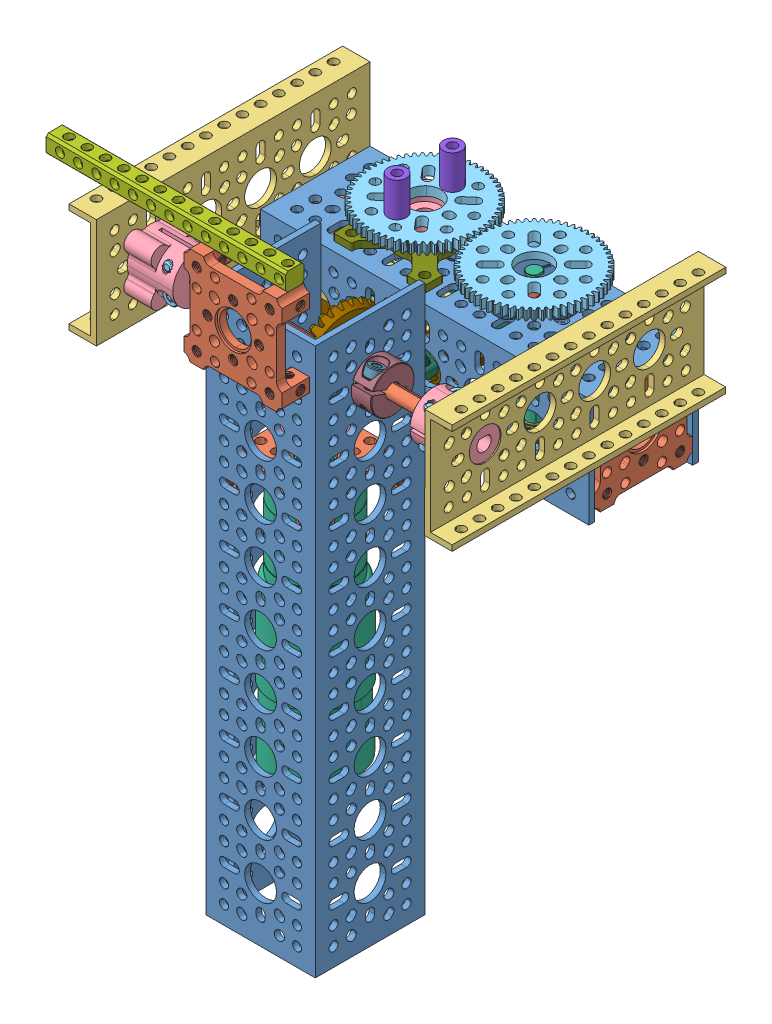
SolidWorks assembly bottom grabber, configuration Default. Lengths in mm.
Overall size (170 269.5 143.08).
60 component instances, 26 part files, 85 mates.
Components (placement in the parent):
- 9 hole u 240mm.step-1: 9 hole u 240mm.step [Default] at (33.7724 45.8602 207.5791) size (48 240 48)
- quad block.step-1: quad block.step [Default] at (33.7724 285.8602 222.0791) x (1 0 0) z (0 1 0) size (43.01 12.01 43.01)
- 4 Hole Low-Side U Channel 120mm.step-1: 4 Hole Low-Side U Channel 120mm.step [Default] at (-62.2276 283.3274 90.0717) x (-1 0 0) z (0 1 -0.000343) size (12 120 48)
- 4 Hole Low-Side U Channel 120mm.step-2: 4 Hole Low-Side U Channel 120mm.step [Default] at (129.7724 240.3274 90.0865) x (1 0 0) z (0 -1 0.000343) size (12 120 48)
- quad block.step-2: quad block.step [Default] at (-38.2276 229.8356 114.0901) x (0 -0.000343 -1) z (0 -1 0.000343) size (43.01 12.01 43.01)
- quad block.step-3: quad block.step [Default] at (105.7724 229.8356 114.0901) x (0 1 -0.000343) z (0 0.000343 1) size (43.01 12.01 43.01)
- 1310-0016-1250 assembly.STEP-1: 1310-0016-1250 assembly.STEP [Default] at (-24.0945 257.948 182.0561) x (0 -1 0.000343) z (0 0.000343 1) size (24 22.55 24)
  - 1310-0016-1250.STEP-1: 1310-0016-1250.STEP [Default] at (-3.9109 -16.1331 4.0243) size (24 22 24)
  - 2800-0004-0012_90128A207.STEP-1: 2800-0004-0012_90128A207.STEP [Default] at (2.0891 1.4669 -4.7257) x (0.720123 -0.693846 0) z (0 0 -1) size (7 7 16.01)
  - 2800-0004-0012_90128A207.STEP-2: 2800-0004-0012_90128A207.STEP [Default] at (-9.9109 1.4669 12.7743) x (-0.720123 -0.693846 0) z (0 0 1) size (7 7 16.01)
- 1310-0016-1250 assembly.STEP-2: 1310-0016-1250 assembly.STEP [Default] at (91.6393 265.8859 189.9886) x (0 0.000343 1) z (0 -1 0.000343) size (24 22.55 24)
  - 1310-0016-1250.STEP-1: 1310-0016-1250.STEP [Default] at (-3.9109 -16.1331 4.0243) size (24 22 24)
  - 2800-0004-0012_90128A207.STEP-1: 2800-0004-0012_90128A207.STEP [Default] at (2.0891 1.4669 -4.7257) x (0.720123 -0.693846 0) z (0 0 -1) size (7 7 16.01)
  - 2800-0004-0012_90128A207.STEP-2: 2800-0004-0012_90128A207.STEP [Default] at (-9.9109 1.4669 12.7743) x (-0.720123 -0.693846 0) z (0 0 1) size (7 7 16.01)
- quad block.step-4: quad block.step [Default] at (33.7724 221.8602 186.0791) x (1 0 0) z (0 0 -1) size (43.01 12.01 43.01)
- motor.step-1: motor.step [Default] at (33.7724 217.8602 186.0791) x (1 0 0) z (0 1 0) size (37.5 37.5 140.7)
- bevel gears.STEP-1: bevel gears.STEP [Default] at (-30.0117 266.7054 228.4687) x (-1 0 0) z (0 0 -1) size (28.77 52.3 42.6)
  - 2306-0006-0014 rev2 assembly.STEP-1: 2306-0006-0014 rev2 assembly.STEP [Default] at (-74.5657 -38.2067 37.2088) x (0 1 0) z (-0.223733 0 0.97465) size (15.33 23.91 24.42)
    - 2306-0006-0014 rev2.STEP-1: 2306-0006-0014 rev2.STEP [Default] at (11.7425 -11.6675 2.6373) size (15.33 23.91 24.42)
    - 2306-0006-0014 rev2 clamp.STEP-1: 2306-0006-0014 rev2 clamp.STEP [Default] at (11.742 -11.6675 2.6373) size (9.55 8.86 18.69)
    - 2800-0004-0012_90128A207.STEP-1: 2800-0004-0012_90128A207.STEP [Default] at (7.1337 -20.4175 7.8873) x (0.998516 0 -0.054455) z (0 -1 0) size (7 7 16.01)
    - 2800-0004-0012_90128A207.STEP-2: 2800-0004-0012_90128A207.STEP [Default] at (7.1337 -20.4175 -2.6127) x (1 0 0) z (0 -1 0) size (7 7 16.01)
  - 2307-0014-0028.STEP-1: 2307-0014-0028.STEP [Default] at (-76.6728 -4.8452 42.3896) size (6.38 42.6 42.6)
- sonic hub.STEP-1: sonic hub.STEP [Default] at (63.9152 236.0435 203.7525) x (0 -0.788084 0.615567) z (-1 0 0) size (28.36 32 9.95)
  - 1311-0016-1006.STEP-1: 1311-0016-1006.STEP [Default] at (-31.225 1.9638 14.6428) size (25.38 32 9)
  - 2800-0004-0014_90128A207.STEP-1: 2800-0004-0014_90128A207.STEP [Default] at (-33.2778 -9.1549 14.6428) x (0.5 -0.5 0.707107) z (-0.707107 -0.707107 0) size (7 7 18.01)
  - 2800-0004-0014_90128A207.STEP-2: 2800-0004-0014_90128A207.STEP [Default] at (-29.1721 13.0826 14.6428) x (-0.5 0.5 0.707107) z (0.707107 0.707107 0) size (7 7 18.01)
- 6mm bearing.step-1: 6mm bearing.step [Default] at (53.7724 261.8602 186.0791) x (0 -0.052204 -0.998636) z (0 -0.998636 0.052204) size (15 5 15)
- 6mm bearing.step-2: 6mm bearing.step [Default] at (13.7724 261.8602 186.0791) x (0 -0.667972 -0.744186) z (0 0.744186 -0.667972) size (15 5 15)
- clamp collar.STEP-1: clamp collar.STEP [Default] at (3.7519 294.0702 171.6983) x (0 0.997254 0.07406) z (0 -0.07406 0.997254) size (19 9.89 19.83)
  - 2910-0919-0006.STEP-1: 2910-0919-0006.STEP [Default] at (-31.0565 -0.5204 16.7268) size (19 9.5 18.97)
  - 2800-0004-0010_90128A207.STEP-1: 2800-0004-0010_90128A207.STEP [Default] at (-24.2865 -0.5204 11.2868) x (0 -0.807243 -0.59022) z (1 0 0) size (7 7 14.01)
- clamp collar.STEP-2: clamp collar.STEP [Default] at (62.7519 238.5667 212.5687) x (0 -0.937484 0.348027) z (0 -0.348027 -0.937484) size (19 9.89 19.83)
  - 2910-0919-0006.STEP-1: 2910-0919-0006.STEP [Default] at (-31.0565 -0.5204 16.7268) size (19 9.5 18.97)
  - 2800-0004-0010_90128A207.STEP-1: 2800-0004-0010_90128A207.STEP [Default] at (-24.2865 -0.5204 11.2868) x (0 -0.807243 -0.59022) z (1 0 0) size (7 7 14.01)
- quad block.step-5: quad block.step [Default] at (57.7724 205.8356 114.0983) x (1 0 0) z (0 0.000343 1) size (43.01 12.01 43.01)
- pattern mount for servo block.step-1: pattern mount for servo block.step [Default] at (9.7724 235.3287 94.0882) x (0 -1 0.000343) z (0 0.000343 1) size (32 38 8.5)
- pattern mount for servo block.step-2: pattern mount for servo block.step [Default] at (9.7724 235.3424 134.0882) x (0 -1 0.000343) z (0 -0.000343 -1) size (32 38 8.5)
- pillow block.STEP-1: pillow block.STEP [Default] at (50.7706 235.1583 107.1797) x (1 0 0) z (0 0.000343 1) size (40 6 40)
  - 1603-0032-0010.STEP-1: 1603-0032-0010.STEP [Default] at (-40.9982 18.675 6.9085) size (40 6 40)
  - 1600-0415-0010.STEP-1: 1600-0415-0010.STEP [Default] at (-40.9982 20.675 6.9085) x (0.898371 0 0.439237) z (-0.439237 0 0.898371) size (15 4 15)
- servo mount plate.step-1: servo mount plate.step [Default] at (0.7724 216.3356 114.0947) x (-1 0 0) z (0 -0.000343 -1) size (63 3.01 40)
- 5 hole u 144mm.step-1: 5 hole u 144mm.step [Default] at (-38.2276 251.3356 114.0827) x (0 0.000343 1) z (0 1 -0.000343) size (48 144 48)
- 140mm dshaft.step-1: 140mm dshaft.step [Default] at (-40.2276 261.8602 186.0791) x (0 -0.581727 -0.813384) z (0 -0.813384 0.581727) size (6 140 5.5)
- servo.step-1: servo.step [Default] at (-0.0776 230.5356 114.0898) x (-1 0 0) z (0 1 -0.000343) size (54.3 20 43.9)
- servo horn-1: servo horn [Default] at (9.7724 265.8356 114.0777) x (-0.075103 0.000342 0.997176) z (0.997176 0.000026 0.075103) size (32 33 32)
- 60 tooth gear.step-1: 60 tooth gear.step [Default] at (9.7724 269.8356 114.0763) x (0.652004 0.00026 0.758216) z (0 -1 0.000343) size (49.6 49.6 4)
- 70mm dshaft.step-1: 70mm dshaft.step [Default] at (57.7724 196.8356 114.1014) x (0.000028 0.000343 1) z (-1 0 0.000028) size (6 70 5.5)
- 6mm bearing.step-3: 6mm bearing.step [Default] at (57.7724 210.8356 114.0966) x (-0.879079 -0.000163 -0.476677) z (-0.476677 0.000301 0.879079) size (15 5 15)
- clamp collar.STEP-3: clamp collar.STEP [Default] at (45.7623 200.8038 80.933) x (-0.74562 -0.000228 -0.666371) z (-0.666371 0.000255 0.74562) size (19 9.89 19.83)
  - 2910-0919-0006.STEP-1: 2910-0919-0006.STEP [Default] at (-31.0565 -0.5204 16.7268) size (19 9.5 18.97)
  - 2800-0004-0010_90128A207.STEP-1: 2800-0004-0010_90128A207.STEP [Default] at (-24.2865 -0.5204 11.2868) x (0 -0.807243 -0.59022) z (1 0 0) size (7 7 14.01)
- sonic hub.STEP-2: sonic hub.STEP [Default] at (78.4638 246.2008 137.5519) x (0.707127 0.000242 0.707087) z (0 1 -0.000343) size (28.36 32 9.95)
  - 1311-0016-1006.STEP-1: 1311-0016-1006.STEP [Default] at (-31.225 1.9638 14.6428) size (25.38 32 9)
  - 2800-0004-0014_90128A207.STEP-1: 2800-0004-0014_90128A207.STEP [Default] at (-33.2778 -9.1549 14.6428) x (0.5 -0.5 0.707107) z (-0.707107 -0.707107 0) size (7 7 18.01)
  - 2800-0004-0014_90128A207.STEP-2: 2800-0004-0014_90128A207.STEP [Default] at (-29.1721 13.0826 14.6428) x (-0.5 0.5 0.707107) z (0.707107 0.707107 0) size (7 7 18.01)
- 60 tooth gear.step-2: 60 tooth gear.step [Default] at (57.7724 268.8356 114.0767) x (0.707087 -0.000242 -0.707127) z (0 -1 0.000343) size (49.6 49.6 4)
- 112mm shaft beam-1: 112mm shaft beam [Default] at (-70.2276 311.3602 214.0791) x (0 -1 0) z (0 0 1) size (8 127 8)
- spacer for claw-1: spacer for claw [Default] at (10.6221 269.8317 102.7946) x (-0.559836 -0.000284 -0.828603) z (0.828603 -0.000192 -0.559836) size (8 15 8)
- spacer for claw-2: spacer for claw [Default] at (8.9227 269.8394 125.3581) x (0.943099 -0.000114 -0.332512) z (0.332512 0.000323 0.943099) size (8 15 8)
Mates (geometry in assembly coordinates):
- Coincident1: coincident anti-aligned: plane of 9 hole u 240mm.step-1 through (57.7724 285.8602 210.0791) normal (0 0 1); plane of quad block.step-1 through (33.7724 285.8602 210.0791) normal (0 0 -1)
- Concentric1: concentric anti-aligned: cylinder of 9 hole u 240mm.step-1 through (49.7724 269.8602 200.0791) axis (0 0 1) radius 2; circle of quad block.step-1
- Parallel1: parallel aligned: plane of 9 hole u 240mm.step-1 through (57.7724 285.8602 162.0791) normal (1 0 0); plane of quad block.step-1 through (55.2724 285.8602 218.0791) normal (1 0 0)
- Concentric2: concentric anti-aligned: cylinder of 9 hole u 240mm.step-1 through (47.7724 261.8602 186.0791) axis (1 0 0) radius 7; circle of 4 Hole Low-Side U Channel 120mm.step-2
- Concentric3: concentric anti-aligned: cylinder of 9 hole u 240mm.step-1 through (19.7724 261.8602 186.0791) axis (-1 0 0) radius 7; circle of 4 Hole Low-Side U Channel 120mm.step-1
- Distance1: distance = 48 mm anti-aligned: plane of 4 Hole Low-Side U Channel 120mm.step-1 through (-38.2276 237.8685 210.0873) normal (1 0 0); plane of 9 hole u 240mm.step-1 through (9.7724 285.8602 162.0791) normal (-1 0 0)
- Coincident8: coincident aligned: plane of 4 Hole Low-Side U Channel 120mm.step-1 through (-86.2276 285.8685 210.0709) normal (0 1 -0.000343); plane of 4 Hole Low-Side U Channel 120mm.step-2 through (108.2724 285.8685 210.0709) normal (0 1 -0.000343)
- Coincident16: coincident: plane of quad block.step-2 through (-47.42 208.3356 114.0974) normal (0 -1 0.000343); plane of quad block.step-3 through (101.7724 208.3356 114.0974) normal (0 -1 0.000343)
- Coincident18: coincident: plane of 4 Hole Low-Side U Channel 120mm.step-1 through (-38.2276 237.8685 210.0873) normal (1 0 0); plane of quad block.step-2 through (-38.2276 229.8356 114.0901) normal (-1 0 0)
- Concentric4: concentric: cylinder of 4 Hole Low-Side U Channel 120mm.step-1 through (-48.2276 245.8301 98.0846) axis (1 0 0) radius 2; circle of quad block.step-2
- Coincident21: coincident: plane of 4 Hole Low-Side U Channel 120mm.step-1 through (-38.2276 237.8685 210.0873) normal (1 0 0); plane of 1310-0016-1250 assembly.STEP-1/1310-0016-1250.STEP-1 through (-38.2276 261.8602 186.0791) normal (-1 0 0)
- Concentric7: concentric: cylinder of 4 Hole Low-Side U Channel 120mm.step-1 through (-48.2276 269.8575 178.0763) axis (1 0 0) radius 2; cylinder of 1310-0016-1250 assembly.STEP-1/1310-0016-1250.STEP-1 through (-18.2276 269.8575 178.0763) axis (-1 0 0) radius 4
- Concentric9: concentric anti-aligned: cylinder of 4 Hole Low-Side U Channel 120mm.step-2 through (115.7724 269.8575 178.0763) axis (-1 0 0) radius 2; cylinder of 1310-0016-1250 assembly.STEP-2/1310-0016-1250.STEP-1 through (85.7724 269.8575 178.0763) axis (1 0 0) radius 4
- Coincident22: coincident anti-aligned: plane of 4 Hole Low-Side U Channel 120mm.step-2 through (105.7724 285.8685 210.0709) normal (-1 0 0); plane of 1310-0016-1250 assembly.STEP-2/1310-0016-1250.STEP-1 through (105.7724 261.8602 186.0791) normal (1 0 0)
- Parallel3: parallel: plane of 9 hole u 240mm.step-1 through (12.2724 285.8602 207.5791) normal (0 0 -1); plane of quad block.step-4 through (33.7724 231.0526 164.5791) normal (0 0 -1)
- Concentric10: concentric: circle of 9 hole u 240mm.step-1; circle of quad block.step-4
- Coincident26: coincident: plane of 9 hole u 240mm.step-1 through (12.2724 285.8602 207.5791) normal (1 0 0); plane of quad block.step-4 through (12.2724 217.8602 186.0791) normal (-1 0 0)
- Concentric11: concentric: circle of quad block.step-4; cylinder of motor.step-1 through (33.7724 136.4602 186.0791) axis (0 1 0) radius 18.75
- Coincident27: coincident: plane of quad block.step-4 through (33.7724 217.8602 186.0791) normal (0 -1 0); plane of motor.step-1 through (33.7724 217.8602 186.0791) normal (0 1 0)
- Concentric12: concentric: cylinder of quad block.step-4 through (25.7724 221.8602 178.0791) axis (0 -1 0) radius 2; circle of motor.step-1
- Concentric14: concentric: cylinder of motor.step-1 through (33.7724 241.8602 186.0791) axis (0 -1 0) radius 3; circle of bevel gears.STEP-1/2306-0006-0014 rev2 assembly.STEP-1/2306-0006-0014 rev2.STEP-1
- Concentric15: concentric: circle of bevel gears.STEP-1/2307-0014-0028.STEP-1; circle of sonic hub.STEP-1/1311-0016-1006.STEP-1
- Coincident31: coincident: plane of bevel gears.STEP-1/2307-0014-0028.STEP-1 through (45.2724 261.8602 186.0791) normal (1 0 0); plane of sonic hub.STEP-1/1311-0016-1006.STEP-1 through (45.2724 261.8602 186.0791) normal (-1 0 0)
- Concentric16: concentric: cylinder of 9 hole u 240mm.step-1 through (47.7724 261.8602 186.0791) axis (1 0 0) radius 7; cylinder of 6mm bearing.step-1 through (57.7724 261.8602 186.0791) axis (-1 0 0) radius 7
- Coincident32: coincident: plane of 9 hole u 240mm.step-1 through (57.7724 285.8602 162.0791) normal (1 0 0); plane of 6mm bearing.step-1 through (57.7724 261.8602 186.0791) normal (-1 0 0)
- Concentric17: concentric anti-aligned: cylinder of 9 hole u 240mm.step-1 through (19.7724 261.8602 186.0791) axis (-1 0 0) radius 7; cylinder of 6mm bearing.step-2 through (9.7724 261.8602 186.0791) axis (1 0 0) radius 7
- Coincident33: coincident anti-aligned: plane of 9 hole u 240mm.step-1 through (9.7724 285.8602 162.0791) normal (-1 0 0); plane of 6mm bearing.step-2 through (9.7724 261.8602 186.0791) normal (1 0 0)
- Coincident34: coincident: plane of 6mm bearing.step-2 through (8.7724 261.8602 186.0791) normal (-1 0 0); plane of clamp collar.STEP-1/2910-0919-0006.STEP-1 through (8.7724 261.8602 186.0791) normal (1 0 0)
- Coincident35: coincident: plane of 6mm bearing.step-1 through (58.7724 261.8602 186.0791) normal (1 0 0); plane of clamp collar.STEP-2/2910-0919-0006.STEP-1 through (58.7724 261.8602 186.0791) normal (-1 0 0)
- Coincident52: coincident anti-aligned: plane of pattern mount for servo block.step-1 through (9.7724 219.3301 98.0936) normal (0 -1 0.000343); plane of servo mount plate.step-1 through (0.7724 219.3356 114.0936) normal (0 1 -0.000343)
- Concentric27: concentric: circle of 4 Hole Low-Side U Channel 120mm.step-2; circle of quad block.step-3
- Coincident59: coincident: plane of 4 Hole Low-Side U Channel 120mm.step-2 through (105.7724 285.8685 210.0709) normal (-1 0 0); plane of quad block.step-3 through (105.7724 229.8356 114.0901) normal (1 0 0)
- Coincident60: coincident: plane of quad block.step-3 through (101.7724 251.3356 114.0827) normal (0 1 -0.000343); plane of 5 hole u 144mm.step-1 through (105.7724 251.3282 92.5827) normal (0 -1 0.000343)
- Coincident61: coincident: plane of quad block.step-2 through (-34.2276 229.8282 92.5901) normal (0 -0.000343 -1); plane of 5 hole u 144mm.step-1 through (105.7724 251.3282 92.5827) normal (0 0.000343 1)
- Distance3: distance = 48 mm anti-aligned: plane of 4 Hole Low-Side U Channel 120mm.step-2 through (105.7724 285.8685 210.0709) normal (-1 0 0); plane of 9 hole u 240mm.step-1 through (57.7724 285.8602 162.0791) normal (1 0 0)
- Coincident63: coincident: plane of quad block.step-3 through (105.7724 229.8356 114.0901) normal (1 0 0); plane of 5 hole u 144mm.step-1 through (105.7724 251.3356 114.0827) normal (1 0 0)
- Concentric28: concentric: circle of 4 Hole Low-Side U Channel 120mm.step-2; circle of quad block.step-3
- Concentric29: concentric: circle of clamp collar.STEP-2/2910-0919-0006.STEP-1; cylinder of 140mm dshaft.step-1 through (99.7724 261.8602 186.0791) axis (-1 0 0) radius 3
- Concentric30: concentric: circle of 1310-0016-1250 assembly.STEP-1/1310-0016-1250.STEP-1; cylinder of 140mm dshaft.step-1 through (99.7724 261.8602 186.0791) axis (-1 0 0) radius 3
- Concentric31: concentric: circle of 6mm bearing.step-1; cylinder of 140mm dshaft.step-1 through (99.7724 261.8602 186.0791) axis (-1 0 0) radius 3
- Concentric32: concentric: circle of sonic hub.STEP-1/1311-0016-1006.STEP-1; cylinder of 140mm dshaft.step-1 through (99.7724 261.8602 186.0791) axis (-1 0 0) radius 3
- Concentric33: concentric: cylinder of clamp collar.STEP-1/2910-0919-0006.STEP-1 through (8.7724 261.8602 186.0791) axis (-1 0 0) radius 9.5; cylinder of 140mm dshaft.step-1 through (99.7724 261.8602 186.0791) axis (-1 0 0) radius 3
- Concentric34: concentric aligned: cylinder of 1310-0016-1250 assembly.STEP-2/1310-0016-1250.STEP-1 through (107.7724 261.8602 186.0791) axis (-1 0 0) radius 3.175; cylinder of 140mm dshaft.step-1 through (99.7724 261.8602 186.0791) axis (-1 0 0) radius 3
- Coincident68: coincident: plane of 1310-0016-1250 assembly.STEP-1/1310-0016-1250.STEP-1 through (-40.2276 261.8602 186.0791) normal (-1 0 0); plane of 140mm dshaft.step-1 through (-40.2276 261.8602 186.0791) normal (-1 0 0)
- Coincident69: coincident: plane of pillow block.STEP-1/1603-0032-0010.STEP-1 through (9.7724 253.8356 114.0818) normal (0 -1 0.000343); plane of 5 hole u 144mm.step-1 through (105.7724 253.8438 138.0818) normal (0 1 -0.000343)
- Concentric35: concentric: circle of pillow block.STEP-1/1603-0032-0010.STEP-1; circle of 5 hole u 144mm.step-1
- Parallel6: parallel: plane of pillow block.STEP-1/1603-0032-0010.STEP-1 through (9.7724 256.8424 134.0808) normal (0 0.000343 1); plane of 5 hole u 144mm.step-1 through (105.7724 205.8438 138.0983) normal (0 0.000343 1)
- Coincident72: coincident anti-aligned: plane of pattern mount for servo block.step-1 through (9.7724 235.3282 92.5882) normal (0 -0.000343 -1); plane of 5 hole u 144mm.step-1 through (105.7724 251.3282 92.5827) normal (0 0.000343 1)
- Coincident73: coincident anti-aligned: plane of pattern mount for servo block.step-2 through (9.7724 235.3429 135.5882) normal (0 0.000343 1); plane of 5 hole u 144mm.step-1 through (105.7724 251.3429 135.5827) normal (0 -0.000343 -1)
- Parallel7: parallel aligned: plane of pattern mount for servo block.step-1 through (9.7724 235.3282 92.5882) normal (0 -0.000343 -1); plane of servo mount plate.step-1 through (0.7724 219.3287 94.0936) normal (0 -0.000343 -1)
- Coincident75: coincident anti-aligned: plane of pattern mount for servo block.step-2 through (9.7724 219.3411 130.0936) normal (0 -1 0.000343); plane of servo mount plate.step-1 through (0.7724 219.3356 114.0936) normal (0 1 -0.000343)
- Coincident76: coincident anti-aligned: circle of pattern mount for servo block.step-1; cylinder of servo mount plate.step-1 through (-6.2276 216.3301 98.0947) axis (0 1 -0.000343) radius 2
- Coincident77: coincident aligned: plane of pattern mount for servo block.step-1 through (-9.2276 235.3301 98.0882) normal (-1 0 0); plane of pattern mount for servo block.step-2 through (-9.2276 235.3411 130.0882) normal (-1 0 0)
- Coincident78: coincident anti-aligned: plane of pattern mount for servo block.step-1 through (9.7724 251.3301 98.0827) normal (0 1 -0.000343); plane of 5 hole u 144mm.step-1 through (105.7724 251.3282 92.5827) normal (0 -1 0.000343)
- Concentric36: concentric: circle of pattern mount for servo block.step-1; circle of pillow block.STEP-1/1603-0032-0010.STEP-1
- Coincident80: coincident: plane of quad block.step-5 through (57.7724 205.8356 114.0983) normal (0 -1 0.000343); plane of 5 hole u 144mm.step-1 through (105.7724 205.8282 92.5983) normal (0 -1 0.000343)
- Concentric37: concentric: circle of quad block.step-5; cylinder of 5 hole u 144mm.step-1 through (73.7724 213.8404 128.0955) axis (0 0.000343 1) radius 2
- Coincident82: coincident: plane of quad block.step-5 through (57.7724 196.6506 135.6014) normal (0 0.000343 1); plane of 5 hole u 144mm.step-1 through (105.7724 251.3429 135.5827) normal (0 -0.000343 -1)
- Concentric38: concentric: cylinder of pillow block.STEP-1/1600-0415-0010.STEP-1 through (9.7724 255.8356 114.0811) axis (0 1 -0.000343) radius 5; cylinder of servo horn-1 through (9.7724 232.8356 114.089) axis (0 1 -0.000343) radius 5
- Coincident83: coincident anti-aligned: plane of servo mount plate.step-1 through (0.7724 219.3356 114.0936) normal (0 1 -0.000343); plane of servo.step-1 through (-25.7276 219.3385 122.5936) normal (0 -1 0.000343)
- Concentric39: concentric: cylinder of pillow block.STEP-1/1600-0415-0010.STEP-1 through (9.7724 255.8356 114.0811) axis (0 1 -0.000343) radius 5; circle of servo.step-1
- Parallel9: parallel anti-aligned: plane of servo mount plate.step-1 through (0.7724 219.332 103.5936) normal (0 0.000343 1); plane of servo.step-1 through (-19.5276 219.3322 104.0936) normal (0 -0.000343 -1)
- Coincident88: coincident: plane of pillow block.STEP-1/1603-0032-0010.STEP-1 through (9.7724 259.8356 114.0798) normal (0 1 -0.000343); plane of servo horn-1 through (9.7724 259.8356 114.0798) normal (0 -1 0.000343)
- Concentric40: concentric anti-aligned: circle of servo horn-1; circle of 60 tooth gear.step-1
- Coincident89: coincident anti-aligned: plane of servo horn-1 through (9.7724 265.8356 114.0777) normal (0 1 -0.000343); plane of 60 tooth gear.step-1 through (-9.0387 265.8409 129.6181) normal (0 -1 0.000343)
- Concentric41: concentric aligned: circle of servo horn-1; circle of 60 tooth gear.step-1
- Concentric43: concentric: circle of 5 hole u 144mm.step-1; cylinder of 70mm dshaft.step-1 through (57.7724 266.8356 114.0774) axis (0 -1 0.000343) radius 3
- Concentric44: concentric: cylinder of quad block.step-5 through (57.7724 205.8356 114.0983) axis (0 1 -0.000343) radius 7; cylinder of 6mm bearing.step-3 through (57.7724 206.8356 114.0979) axis (0 1 -0.000343) radius 7
- Coincident91: coincident: plane of quad block.step-5 through (57.7724 206.8356 114.0979) normal (0 -1 0.000343); plane of 6mm bearing.step-3 through (57.7724 206.8356 114.0979) normal (0 1 -0.000343)
- Concentric45: concentric anti-aligned: cylinder of 6mm bearing.step-3 through (57.7724 210.8356 114.0966) axis (0 -1 0.000343) radius 3; cylinder of clamp collar.STEP-3/2910-0919-0006.STEP-1 through (57.7724 196.8356 114.1014) axis (0 1 -0.000343) radius 3
- Coincident93: coincident anti-aligned: plane of 6mm bearing.step-3 through (57.7724 205.8356 114.0983) normal (0 -1 0.000343); plane of clamp collar.STEP-3/2910-0919-0006.STEP-1 through (57.7724 205.8356 114.0983) normal (0 1 -0.000343)
- Coincident94: coincident: plane of 70mm dshaft.step-1 through (57.7724 196.8356 114.1014) normal (0 -1 0.000343); plane of clamp collar.STEP-3/2910-0919-0006.STEP-1 through (57.7724 196.8356 114.1014) normal (0 -1 0.000343)
- Coincident96: coincident: cylinder of 70mm dshaft.step-1 through (57.7724 266.8356 114.0774) axis (0 -1 0.000343) radius 3; circle of sonic hub.STEP-2/1311-0016-1006.STEP-1
- Parallel10: parallel: plane of 70mm dshaft.step-1 through (60.2724 266.8356 114.0773) normal (1 0 -0.000028); plane of sonic hub.STEP-2/1311-0016-1006.STEP-1 through (60.2524 256.5851 114.0808) normal (-1 0 0.000028)
- Distance6: distance = 3 mm: plane of sonic hub.STEP-2/1311-0016-1006.STEP-1 through (57.7724 256.8356 114.0808) normal (0 -1 0.000343); plane of 5 hole u 144mm.step-1 through (105.7724 253.8438 138.0818) normal (0 1 -0.000343)
- Concentric46: concentric: circle of sonic hub.STEP-2/1311-0016-1006.STEP-1; circle of 60 tooth gear.step-2
- Coincident100: coincident: plane of sonic hub.STEP-2/1311-0016-1006.STEP-1 through (57.7724 264.8356 114.0781) normal (0 1 -0.000343); plane of 60 tooth gear.step-2 through (74.6821 264.8416 131.6684) normal (0 -1 0.000343)
- Concentric47: concentric: cylinder of sonic hub.STEP-2/1311-0016-1006.STEP-1 through (69.0861 249.7951 114.0829) axis (0 1 -0.000343) radius 2; circle of 60 tooth gear.step-2
- Coincident103: coincident anti-aligned: plane of quad block.step-1 through (33.7724 307.3602 231.2715) normal (0 1 0); plane of 112mm shaft beam-1 through (-66.2276 307.3602 214.0791) normal (0 -1 0)
- Concentric48: concentric aligned: circle of quad block.step-1; circle of 112mm shaft beam-1
- Parallel11: parallel aligned: plane of quad block.step-1 through (33.7724 285.8602 222.0791) normal (0 0 1); plane of 112mm shaft beam-1 through (-66.2276 311.3602 218.0791) normal (0 0 1)
- Concentric49: concentric aligned: cylinder of 60 tooth gear.step-1 through (10.6221 269.8317 102.7946) axis (0 -1 0.000343) radius 2; cylinder of spacer for claw-1 through (10.6221 284.8317 102.7895) axis (0 -1 0.000343) radius 2
- Coincident106: coincident anti-aligned: plane of 60 tooth gear.step-1 through (-9.0387 269.8409 129.6167) normal (0 1 -0.000343); plane of spacer for claw-1 through (10.6221 269.8317 102.7946) normal (0 -1 0.000343)
- Concentric50: concentric anti-aligned: cylinder of 60 tooth gear.step-1 through (8.9227 269.8394 125.3581) axis (0 -1 0.000343) radius 2; circle of spacer for claw-2
- Coincident108: coincident anti-aligned: plane of 60 tooth gear.step-1 through (-9.0387 269.8409 129.6167) normal (0 1 -0.000343); plane of spacer for claw-2 through (8.9227 269.8394 125.3581) normal (0 -1 0.000343)
